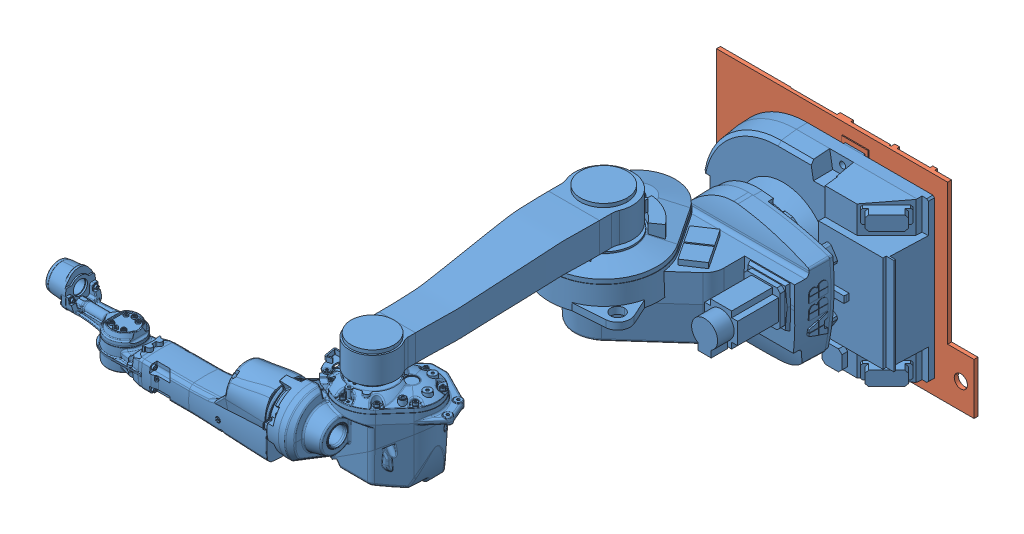
SolidWorks assembly 机器人+工件台, configuration 默认. Lengths in mm.
Overall size (1471.91 580 1415).
2 component instances, 2 part files, 5 mates.
Components (placement in the parent):
- IRB1600ID_4_150__02_STEP_c-1: IRB1600ID_4_150__02_STEP_c [默认] at (-101.9143 0.2591 3) x (-1 0 0) z (0 0 1) size (1372.28 510.23 1392)
- 工件台-2: 工件台 [默认] at (-50 0 -20) x (1 0 0) z (0 -1 0) size (780 23 580)
Mates (geometry in assembly coordinates):
- 重合4: coincident anti-aligned: line of 工件台-2 through (-400 290 0) axis (0 -1 0); line of assembly
- 重合5: coincident aligned: line of 工件台-2 through (-400 -290 0) axis (1 0 0); line of assembly
- 距离1: distance = 8 mm anti-aligned: plane of 工件台-2 through (-50 0 0) normal (0 0 1); plane of IRB1600ID_4_150__02_STEP_c-1 through (-116.9143 0.2591 8) normal (0 0 -1)
- 相切1: tangent: face of IRB1600ID_4_150__02_STEP_c-1; cylinder of 工件台-2 through (-351.9143 0.2591 -20) axis (0 0 1) radius 9.25
- 相切2: tangent: face of IRB1600ID_4_150__02_STEP_c-1; cylinder of 工件台-2 through (23.0857 -216.2472 -15) axis (0 0 1) radius 9.25
